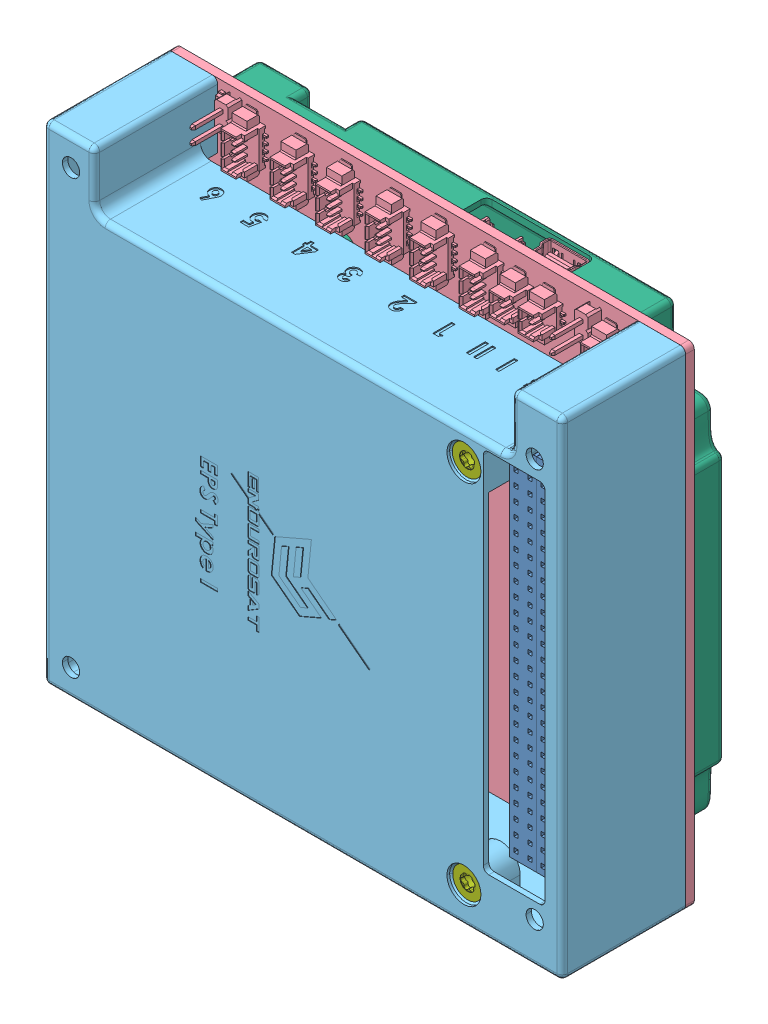
SolidWorks assembly EPS1+, configuration Default. Lengths in mm.
Overall size (95.9 90.21 30).
16 component instances, 8 part files, 0 mates.
Components (placement in the parent):
- EPS1+.STEP-1: EPS1+.STEP [Default] at origin size (95.9 90.21 30)
  - ESQ_126_69_G_D.STEP-1: ESQ_126_69_G_D.STEP [Default] at (61.6205 47.1532 90.3532) x (0 -1 0) z (-1 0 0) size (66.55 23.24 5.08)
    - _ESQ_126_69_G_D_socket_2.STEP-1: _ESQ_126_69_G_D_socket_2.STEP [Default] at (-33.274 0 0) size (66.55 8.51 4.95)
    - _ESQ_126_69_G_D_pins_4.STEP-1: _ESQ_126_69_G_D_pins_4.STEP [Default] at origin size (65.79 19.68 4.7)
    - _ESQ_126_69_G_D_LL_bpins_6.STEP-1: _ESQ_126_69_G_D_LL_bpins_6.STEP [Default] at (-33.147 -10.16 0) size (66.04 10.16 5.08)
  - ESQ_126_69_G_D.STEP-2: ESQ_126_69_G_D.STEP [Default] at (66.637 47.1532 90.3532) x (0 1 0) z (1 0 0) size (66.55 23.24 5.08)
    - _ESQ_126_69_G_D_socket_2.STEP-1: _ESQ_126_69_G_D_socket_2.STEP [Default] at (-33.274 0 0) size (66.55 8.51 4.95)
    - _ESQ_126_69_G_D_pins_4.STEP-1: _ESQ_126_69_G_D_pins_4.STEP [Default] at origin size (65.79 19.68 4.7)
    - _ESQ_126_69_G_D_LL_bpins_6.STEP-1: _ESQ_126_69_G_D_LL_bpins_6.STEP [Default] at (-33.147 -10.16 0) size (66.04 10.16 5.08)
  - ES_EPS_Rev1_4_PCB_STEP.STEP-1: ES_EPS_Rev1_4_PCB_STEP.STEP [Default] at (-22.8876 2.7023 80.1932) size (95.9 90.21 13.97)
  - top-cover.STEP-1: top-cover.STEP [Default] at (-22.8876 2.7023 80.1932) size (95.9 90.2 22.8)
  - bottom-cover_Rev1.2.STEP-1: bottom-cover_Rev1.2.STEP [Default] at (25.0624 47.8023 72.9932) size (95.9 90.2 13.5)
  - 965 M3x6 Torx_M3X6mm.STEP-1: 965 M3x6 Torx_M3X6mm.STEP [Default] at (54.8324 9.3023 102.3047) x (-0.142927 0.989733 0) z (0 0 1) size (5.5 5.5 6)
  - 965 M3x6 Torx_M3X6mm.STEP-2: 965 M3x6 Torx_M3X6mm.STEP [Default] at (54.8324 77.0023 102.394) x (0.179192 -0.983814 0) z (0 0 1) size (5.5 5.5 6)
  - TR Fastenings Ltd-M2_5X4mm.STEP-1: TR Fastenings Ltd-M2_5X4mm.STEP [Default] at (-22.8876 68.8523 83.4832) x (0 0.503629 0.86392) z (-1 0 0) size (4.7 4.7 4)
  - TR Fastenings Ltd-M2_5X4mm.STEP-2: TR Fastenings Ltd-M2_5X4mm.STEP [Default] at (-22.8876 26.7523 83.4832) x (0 -0.360323 0.932827) z (-1 0 0) size (4.7 4.7 4)
